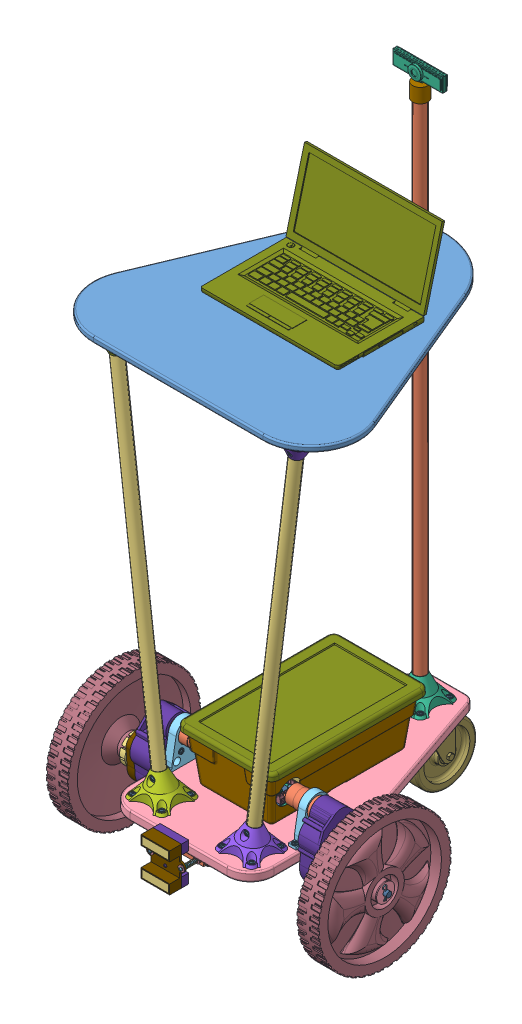
SolidWorks assembly Layla, configuration Default. Lengths in mm. (continued)
Components (placement in the parent): (continued)
- Charger-1: Charger [Default] at (-0.0002 -30.6395 1534.0575) x (1 0 0.000005) z (-0.000005 0 1) size (116 80 70.35)
  - Charger_Back-1: Charger_Back [Default] at (-18.6044 2.3885 -23.0376) size (60 80 15)
  - Charger_Front_1-1: Charger_Front_1 [Default] at (-2.2754 24.6395 -8.0376) x (1 0 0) z (0 -1 0) size (80 25 80)
  - Charger_Front_2-1: Charger_Front_2 [Default] at (-2.2754 54.6395 -6.0376) x (1 0 0) z (0 -1 0) size (54 22 14)
  - Charger_Front_2-2: Charger_Front_2 [Default] at (-2.2754 -5.3605 15.9624) x (1 0 0) z (0 1 0) size (54 22 14)
  - Charge_Bracket-1: Charge_Bracket [Default] at (0 24.6395 -40.9868) x (1 0 0) z (0 1 0) size (116 10 12)
  - Charge_Plate-1: Charge_Plate [Default] at (-2.2754 -5.3605 16.9624) x (-1 0 0) z (0 -1 0) size (56 24 16)
  - Charge_Plate-2: Charge_Plate [Default] at (-2.2754 54.6395 16.9624) x (1 0 0) z (0 1 0) size (56 24 16)
  - Charger_Washer_10-1: Charger_Washer_10 [Default] at (-32.2754 24.6395 -2.5898) x (1 0 0) z (0 1 0) size (12.57 1.45 12.57)
  - Charger_Bolt_6_(2.0'')-1: Charger_Bolt_6_(2.0'') [Default] at (-32.2754 24.6395 -53.3898) x (0 1 0) z (1 0 0) size (6.6 54.26 6.6)
  - Charger_Nut_6-1: Charger_Nut_6 [Default] at (-32.2754 24.6395 -12.4826) x (0 -1 0) z (-1 0 0) size (7.87 4.45 7.87)
  - Charger_Spring-1: Charger_Spring [Default] at (-32.2754 24.6395 -12.7475) x (0.535047 0.844822 0) z (-0.844822 0.535047 0) size (8.88 22.59 8.88)
  - Charger_Washer_10-2: Charger_Washer_10 [Default] at (-32.2754 24.6395 -35.9868) x (0.916814 0.399313 0) z (0.399313 -0.916814 0) size (12.57 1.45 12.57)
  - Charger_Nut_6-2: Charger_Nut_6 [Default] at (-32.2754 24.6395 -45.9868) x (1 0 0) z (0 1 0) size (7.87 4.45 7.87)
  - Charger_Washer_10-3: Charger_Washer_10 [Default] at (32.2754 24.6395 -35.9868) x (-0.916814 0.399313 0) z (0.399313 0.916814 0) size (12.57 1.45 12.57)
  - Charger_Nut_6-3: Charger_Nut_6 [Default] at (32.2754 24.6395 -45.9868) x (-1 0 0) z (0 -1 0) size (7.87 4.45 7.87)
  - Charger_Spring-2: Charger_Spring [Default] at (32.2754 24.6395 -34.274) x (0.535047 -0.844822 0) z (-0.844822 -0.535047 0) size (8.88 22.59 8.88)
  - Charger_Nut_6-4: Charger_Nut_6 [Default] at (32.2754 24.6395 -12.4826) x (0 -1 0) z (-1 0 0) size (7.87 4.45 7.87)
  - Charger_Bolt_6_(2.0'')-2: Charger_Bolt_6_(2.0'') [Default] at (32.2754 24.6395 -53.3898) x (0 1 0) z (1 0 0) size (6.6 54.26 6.6)
  - Charger_Washer_10-4: Charger_Washer_10 [Default] at (32.2754 24.6395 -2.5898) x (-1 0 0) z (0 -1 0) size (12.57 1.45 12.57)
  - Charger_Bolt_Small-1: Charger_Bolt_Small [Default] at (-2.2754 36.6395 -17.7376) x (1 0 0) z (0 -1 0) size (6.1 16.05 6.1)
  - Charger_Bolt_Small-2: Charger_Bolt_Small [Default] at (-2.2754 12.6395 -17.7376) x (1 0 0) z (0 -1 0) size (6.1 16.05 6.1)
- Screw_8_(0.75'')-42: Screw_8_(0.75'') [Default] at (-52 6.7 1493.0704) x (-1 0 0) z (0 0 1) size (10.85 21.85 10.85)
- Screw_8_(0.75'')-43: Screw_8_(0.75'') [Default] at (52 6.7 1493.071) x (-1 0 0) z (0 0 1) size (10.85 21.85 10.85)
Mates (geometry in assembly coordinates):
- Coincident24: coincident anti-aligned: circle of Layla_Bottom-1; circle of frame_bracket_volcano_back-2
- Coincident25: coincident anti-aligned: circle of Layla_Bottom-1; circle of frame_bracket_volcano_back-2
- Coincident27: coincident anti-aligned: plane of Conduit_Back-1 through (0.0274 19.05 997.2192) normal (0 -1 0); plane of Layla_Bottom-1 through (-101.5998 19.05 1455.2076) normal (0 1 0)
- Concentric21: concentric anti-aligned: circle of Conduit_Back-1; circle of Layla_Bottom-1
- Concentric81: concentric anti-aligned: circle of Layla_Top-1; circle of frame_bracket_volcano_back-1
- Coincident75: coincident anti-aligned: plane of Layla_Top-1 through (0.0268 830.9031 1092.4746) normal (0 -1 0); plane of frame_bracket_volcano_back-1 through (0.0274 830.9031 997.2192) normal (0 1 0)
- Concentric83: concentric anti-aligned: circle of Layla_Top-1; circle of frame_bracket_volcano_back-1
- Coincident80: coincident anti-aligned: axis of Conduit_Back-1 through (0.0274 19.05 997.2192) axis (0 1 0); axis of frame_bracket_volcano_back-1 through (0.0274 809.7628 997.2192) axis (0 -1 0)
- Parallel28: parallel aligned: line of Layla_Top-1 through (-0.0833 830.9031 1505.2246) axis (0 0 -1); line of Layla_Bottom-1 through (0 19.05 1501.2457) axis (0 0 -1)
- Coincident89: coincident anti-aligned: circle of Layla_Bottom-1; circle of motor_bracket-1
- Coincident90: coincident aligned: circle of Layla_Bottom-1; circle of motor_bracket-1
- Coincident91: coincident anti-aligned: circle of Layla_Bottom-1; circle of motor_bracket-2
- Coincident92: coincident aligned: circle of Layla_Bottom-1; circle of motor_bracket-2
- Concentric84: concentric aligned: circle of Conduit_Back-1; circle of Camera_Bracket-1
- Coincident94: coincident anti-aligned: plane of Conduit_Back-1 through (0.0274 1136.65 997.2192) normal (0 1 0); plane of Camera_Bracket-1 through (0.0274 1136.65 997.2192) normal (0 -1 0)
- Concentric86: concentric aligned: circle of Layla_Bottom-1; circle of frame_bracket_volcano_right-1
- Concentric87: concentric aligned: circle of Layla_Bottom-1; circle of frame_bracket_volcano_right-1
- Coincident104: coincident anti-aligned: plane of Layla_Bottom-1 through (-101.5998 19.05 1455.2076) normal (0 1 0); plane of frame_bracket_volcano_right-1 through (-94.2631 19.05 1445.5525) normal (0 -1 0)
- Concentric88: concentric aligned: circle of Layla_Bottom-1; circle of frame_bracket_volcano_left-1
- Concentric89: concentric aligned: circle of Layla_Bottom-1; circle of frame_bracket_volcano_left-1
- Coincident105: coincident anti-aligned: plane of Layla_Bottom-1 through (-101.5998 19.05 1455.2076) normal (0 1 0); plane of frame_bracket_volcano_left-1 through (94.2631 19.05 1445.5525) normal (0 -1 0)
- Coincident106: coincident aligned: circle of Conduit_Front-1; circle of frame_bracket_volcano_left-1
- Coincident107: coincident aligned: circle of Conduit_Front-2; circle of frame_bracket_volcano_right-1
- Coincident108: coincident anti-aligned: axis of Conduit_Front-2 through (-94.5769 21.6058 1445.5526) axis (-0.121869 0.992546 0.000001); axis of frame_bracket_volcano_right-1 through (-100.3565 68.6773 1445.5526) axis (0.121869 -0.992546 -0.000001)
- Coincident109: coincident anti-aligned: axis of Conduit_Front-1 through (94.5769 21.6058 1445.5526) axis (0.121869 0.992546 0.000001); axis of frame_bracket_volcano_left-1 through (100.3565 68.6773 1445.5526) axis (-0.121869 -0.992546 -0.000001)
- Coincident110: coincident anti-aligned: circle of Conduit_Front-2; circle of frame_bracket_volcano_right-2
- Coincident111: coincident aligned: axis of Conduit_Front-2 through (-94.5769 21.6058 1445.5526) axis (-0.121869 0.992546 0.000001); axis of frame_bracket_volcano_right-2 through (-187.8526 781.2758 1445.5534) axis (-0.121869 0.992546 0.000001)
- Coincident112: coincident anti-aligned: circle of Conduit_Front-1; circle of frame_bracket_volcano_left-2
- Coincident113: coincident aligned: axis of Conduit_Front-1 through (94.5769 21.6058 1445.5526) axis (0.121869 0.992546 0.000001); axis of frame_bracket_volcano_left-2 through (187.8526 781.2758 1445.5534) axis (0.121869 0.992546 0.000001)
- Coincident114: coincident anti-aligned: plane of Layla_Top-1 through (0.0268 830.9031 1092.4746) normal (0 -1 0); plane of frame_bracket_volcano_left-2 through (193.9461 830.9031 1445.5534) normal (0 1 0)
- Concentric91: concentric aligned: circle of Axle_7_16-2; circle of axle_bracket_7_16-1
- Parallel34: parallel anti-aligned: plane of Layla_Bottom-1 through (-101.5998 0 1455.2076) normal (0 -1 0); plane of axle_bracket_7_16-1 through (74.0819 -2.9787 1334.7553) normal (0 1 0)
- Coincident124: coincident anti-aligned: line of Layla_Bottom-1 through (36.5029 0 951.0085) axis (-0.000005 0 1); line of Caster Part-1 through (36.5024 0 1043.0085) axis (0.000005 0 -1)
- Coincident125: coincident aligned: line of Layla_Bottom-1 through (-36.4971 0 951.0081) axis (-0.000005 0 1); line of Caster Part-1 through (-36.4971 0 951.0081) axis (-0.000005 0 1)
- Coincident126: coincident aligned: line of Layla_Bottom-1 through (36.5029 0 951.0085) axis (-1 0 -0.000005); line of Caster Part-1 through (36.5029 0 951.0085) axis (-1 0 -0.000005)
- Coincident188: coincident aligned: plane of Laptop-2 through (0 841.3074 1314.5854) normal (1 0 0); plane of assembly through (0 0 0) normal (1 0 0)
- Coincident189: coincident anti-aligned: plane of Layla_Top-1 through (0.0268 843.6031 1092.4746) normal (0 1 0); plane of Laptop-2 through (220.359 843.6031 1126.8803) normal (0 -1 0)
- Coincident191: coincident anti-aligned: plane of Caster Part-1 through (176.8474 -3.048 944.9392) normal (0 -1 0); plane of Screw_8_(0.75'')-1 through (-22.2101 -3.048 1035.0706) normal (0 1 0)
- Concentric140: concentric aligned: circle of Caster Part-1; circle of Screw_8_(0.75'')-1
- Parallel92: parallel anti-aligned: plane of Screw_8_(0.75'')-1; plane of assembly through (0 0 0) normal (1 0 0)
- Coincident193: coincident anti-aligned: plane of Caster Part-1 through (176.8474 -3.048 944.9392) normal (0 -1 0); plane of Screw_8_(0.75'')-2 through (22.2149 -3.048 1035.0709) normal (0 1 0)
- Parallel93: parallel anti-aligned: plane of Screw_8_(0.75'')-2; plane of assembly through (0 0 0) normal (1 0 0)
- Concentric141: concentric anti-aligned: circle of Caster Part-1; circle of Screw_8_(0.75'')-2
- Coincident194: coincident anti-aligned: plane of Caster Part-1 through (176.8474 -3.048 944.9392) normal (0 -1 0); plane of Screw_8_(0.75'')-3 through (22.2153 -3.048 958.9459) normal (0 1 0)
- Parallel94: parallel anti-aligned: plane of Screw_8_(0.75'')-3; plane of assembly through (0 0 0) normal (1 0 0)
- Concentric142: concentric aligned: circle of Caster Part-1; circle of Screw_8_(0.75'')-3
- Coincident195: coincident anti-aligned: plane of Caster Part-1 through (176.8474 -3.048 944.9392) normal (0 -1 0); plane of Screw_8_(0.75'')-4 through (-22.2097 -3.048 958.9456) normal (0 1 0)
- Parallel95: parallel anti-aligned: plane of Screw_8_(0.75'')-4; plane of assembly through (0 0 0) normal (1 0 0)
- Concentric143: concentric anti-aligned: circle of Caster Part-1; circle of Screw_8_(0.75'')-4
- Parallel96: parallel anti-aligned: plane of Screw_8_(0.75'')-5; plane of assembly through (0 0 0) normal (1 0 0)
- Coincident196: coincident anti-aligned: plane of axle_bracket_7_16-1 through (82.3318 -5.1787 1347.2554) normal (0 -1 0); plane of Screw_8_(0.75'')-5 through (82.3319 -5.1787 1341.0054) normal (0 1 0)
- Concentric144: concentric aligned: circle of axle_bracket_7_16-1; circle of Screw_8_(0.75'')-5
- Parallel98: parallel anti-aligned: plane of Screw_8_(0.75'')-7; plane of assembly through (0 0 0) normal (1 0 0)
- Coincident198: coincident anti-aligned: plane of axle_bracket_7_16-2 through (-82.3304 -5.1787 1375.5668) normal (0 -1 0); plane of Screw_8_(0.75'')-7 through (-82.3303 -5.1787 1373.3168) normal (0 1 0)
- Concentric146: concentric anti-aligned: circle of axle_bracket_7_16-2; circle of Screw_8_(0.75'')-7
- Parallel100: parallel anti-aligned: plane of Screw_8_(0.75'')-9 through (124.3148 10.35 1475.6049) normal (-1 0 0); plane of assembly through (0 0 0) normal (1 0 0)
- Coincident200: coincident anti-aligned: plane of frame_bracket_volcano_left-1 through (124.3148 23.05 1477.8549) normal (0 1 0); plane of Screw_8_(0.75'')-9 through (124.3148 23.05 1475.6049) normal (0 -1 0)
- Concentric148: concentric aligned: circle of frame_bracket_volcano_left-1; circle of Screw_8_(0.75'')-9
- Parallel101: parallel anti-aligned: plane of Screw_8_(0.75'')-10 through (124.3154 10.35 1415.5008) normal (-1 0 0); plane of assembly through (0 0 0) normal (1 0 0)
- Concentric149: concentric aligned: circle of frame_bracket_volcano_left-1; circle of Screw_8_(0.75'')-10
- Coincident202: coincident anti-aligned: plane of frame_bracket_volcano_left-1 through (124.3153 23.05 1417.7508) normal (0 1 0); plane of Screw_8_(0.75'')-10 through (124.3154 23.05 1415.5008) normal (0 -1 0)
- Parallel102: parallel anti-aligned: plane of Screw_8_(0.75'')-11 through (64.2113 10.35 1415.5002) normal (-1 0 0); plane of assembly through (0 0 0) normal (1 0 0)
- Concentric150: concentric aligned: circle of frame_bracket_volcano_left-1; circle of Screw_8_(0.75'')-11
- Coincident204: coincident anti-aligned: plane of frame_bracket_volcano_left-1 through (64.2113 23.05 1417.7502) normal (0 1 0); plane of Screw_8_(0.75'')-11 through (64.2113 23.05 1415.5002) normal (0 -1 0)
- Parallel103: parallel anti-aligned: plane of Screw_8_(0.75'')-12 through (64.2107 10.35 1475.6043) normal (-1 0 0); plane of assembly through (0 0 0) normal (1 0 0)
- Coincident205: coincident anti-aligned: plane of frame_bracket_volcano_left-1 through (64.2107 23.05 1477.8543) normal (0 1 0); plane of Screw_8_(0.75'')-12 through (64.2107 23.05 1475.6043) normal (0 -1 0)
- Concentric151: concentric aligned: circle of frame_bracket_volcano_left-1; circle of Screw_8_(0.75'')-12
- Parallel104: parallel anti-aligned: plane of Screw_8_(0.75'')-13 through (-64.2107 10.35 1475.6043) normal (-1 0 0); plane of assembly through (0 0 0) normal (1 0 0)
- Coincident206: coincident anti-aligned: plane of frame_bracket_volcano_right-1 through (-64.2107 23.05 1477.8543) normal (0 1 0); plane of Screw_8_(0.75'')-13 through (-64.2107 23.05 1475.6043) normal (0 -1 0)
- Concentric152: concentric anti-aligned: circle of frame_bracket_volcano_right-1; circle of Screw_8_(0.75'')-13
- Parallel105: parallel anti-aligned: plane of Screw_8_(0.75'')-14 through (-124.3148 10.35 1475.6049) normal (-1 0 0); plane of assembly through (0 0 0) normal (1 0 0)
- Coincident208: coincident anti-aligned: plane of frame_bracket_volcano_right-1 through (-124.3148 23.05 1477.8549) normal (0 1 0); plane of Screw_8_(0.75'')-14 through (-124.3148 23.05 1475.6049) normal (0 -1 0)
- Concentric153: concentric anti-aligned: circle of frame_bracket_volcano_right-1; circle of Screw_8_(0.75'')-14
- Parallel106: parallel anti-aligned: plane of Screw_8_(0.75'')-15 through (-124.3154 10.35 1415.5008) normal (-1 0 0); plane of assembly through (0 0 0) normal (1 0 0)
- Coincident209: coincident anti-aligned: plane of frame_bracket_volcano_right-1 through (-124.3153 23.05 1417.7508) normal (0 1 0); plane of Screw_8_(0.75'')-15 through (-124.3154 23.05 1415.5008) normal (0 -1 0)
- Concentric154: concentric anti-aligned: circle of frame_bracket_volcano_right-1; circle of Screw_8_(0.75'')-15
- Parallel108: parallel anti-aligned: plane of Screw_8_(0.75'')-17 through (-64.2113 10.35 1415.5002) normal (-1 0 0); plane of assembly through (0 0 0) normal (1 0 0)
- Coincident211: coincident anti-aligned: plane of frame_bracket_volcano_right-1 through (-64.2113 23.05 1417.7502) normal (0 1 0); plane of Screw_8_(0.75'')-17 through (-64.2113 23.05 1415.5002) normal (0 -1 0)
- Concentric156: concentric anti-aligned: circle of frame_bracket_volcano_right-1; circle of Screw_8_(0.75'')-17
- Parallel109: parallel anti-aligned: plane of Screw_8_(0.75'')-18 through (-136.3198 11.314 1395.7818) normal (-1 0 0); plane of assembly through (0 0 0) normal (1 0 0)
- Coincident212: coincident anti-aligned: plane of motor_bracket-2 through (-136.3143 24.014 1395.7771) normal (0 1 0); plane of Screw_8_(0.75'')-18 through (-136.3198 24.014 1395.7818) normal (0 -1 0)
- Concentric157: concentric anti-aligned: circle of motor_bracket-2; circle of Screw_8_(0.75'')-18
- Parallel110: parallel anti-aligned: plane of Screw_8_(0.75'')-19 through (-136.3202 11.314 1318.2818) normal (-1 0 0); plane of assembly through (0 0 0) normal (1 0 0)
- Coincident213: coincident anti-aligned: plane of motor_bracket-2 through (-136.3147 24.014 1318.2866) normal (0 1 0); plane of Screw_8_(0.75'')-19 through (-136.3202 24.014 1318.2818) normal (0 -1 0)
- Concentric158: concentric aligned: circle of motor_bracket-2; circle of Screw_8_(0.75'')-19
- Parallel111: parallel anti-aligned: plane of Screw_8_(0.75'')-20 through (136.3198 11.314 1395.7818) normal (-1 0 0); plane of assembly through (0 0 0) normal (1 0 0)
- Coincident214: coincident anti-aligned: plane of motor_bracket-1 through (136.3143 24.014 1395.7771) normal (0 1 0); plane of Screw_8_(0.75'')-20 through (136.3198 24.014 1395.7818) normal (0 -1 0)
- Concentric159: concentric aligned: circle of motor_bracket-1; circle of Screw_8_(0.75'')-20
- Parallel112: parallel anti-aligned: plane of Screw_8_(0.75'')-21 through (136.3202 11.314 1318.2818) normal (-1 0 0); plane of assembly through (0 0 0) normal (1 0 0)
- Coincident215: coincident anti-aligned: plane of motor_bracket-1 through (136.3147 24.014 1318.2866) normal (0 1 0); plane of Screw_8_(0.75'')-21 through (136.3202 24.014 1318.2818) normal (0 -1 0)
- Concentric160: concentric anti-aligned: circle of motor_bracket-1; circle of Screw_8_(0.75'')-21
- Parallel113: parallel anti-aligned: plane of Screw_8_(0.75'')-22 through (30.0513 10.35 1027.3271) normal (-1 0 0); plane of assembly through (0 0 0) normal (1 0 0)
- Coincident216: coincident anti-aligned: plane of frame_bracket_volcano_back-2 through (30.0491 23.05 1025.0771) normal (0 1 0); plane of Screw_8_(0.75'')-22 through (30.0513 23.05 1027.3271) normal (0 -1 0)
- Concentric161: concentric anti-aligned: circle of frame_bracket_volcano_back-2; circle of Screw_8_(0.75'')-22
- Parallel114: parallel anti-aligned: plane of Screw_8_(0.75'')-23 through (29.9912 10.35 967.223) normal (-1 0 0); plane of assembly through (0 0 0) normal (1 0 0)
- Coincident217: coincident anti-aligned: plane of frame_bracket_volcano_back-2 through (29.9889 23.05 964.973) normal (0 1 0); plane of Screw_8_(0.75'')-23 through (29.9912 23.05 967.223) normal (0 -1 0)
- Concentric162: concentric anti-aligned: circle of frame_bracket_volcano_back-2; circle of Screw_8_(0.75'')-23
- Parallel115: parallel anti-aligned: plane of Screw_8_(0.75'')-24 through (-30.1129 10.35 967.2832) normal (-1 0 0); plane of assembly through (0 0 0) normal (1 0 0)
- Coincident218: coincident anti-aligned: plane of frame_bracket_volcano_back-2 through (-30.1151 23.05 965.0332) normal (0 1 0); plane of Screw_8_(0.75'')-24 through (-30.1129 23.05 967.2832) normal (0 -1 0)
- Concentric163: concentric anti-aligned: circle of frame_bracket_volcano_back-2; circle of Screw_8_(0.75'')-24
- Parallel116: parallel anti-aligned: plane of Screw_8_(0.75'')-25 through (-30.0527 10.35 1027.3872) normal (-1 0 0); plane of assembly through (0 0 0) normal (1 0 0)
- Coincident219: coincident anti-aligned: plane of frame_bracket_volcano_back-2 through (-30.055 23.05 1025.1372) normal (0 1 0); plane of Screw_8_(0.75'')-25 through (-30.0527 23.05 1027.3872) normal (0 -1 0)
- Concentric164: concentric anti-aligned: circle of frame_bracket_volcano_back-2; circle of Screw_8_(0.75'')-25
- Coincident222: coincident anti-aligned: plane of frame_bracket_volcano_back-2 through (-0.0446 50.3 983.4551) normal (-0.001001 0 -0.999999); plane of Screw_8_(0.75'')-28 through (-0.0446 56.55 983.4551) normal (0.001001 0 0.999999)
- Concentric167: concentric aligned: circle of frame_bracket_volcano_back-2; circle of Screw_8_(0.75'')-28
- Parallel121: parallel aligned: plane of Layla_Bottom-1 through (-101.5998 19.05 1455.2076) normal (0 1 0); plane of Screw_8_(0.75'')-28
- Coincident225: coincident anti-aligned: plane of frame_bracket_volcano_left-1 through (103.0472 51.655 1459.4026) normal (-0.000009 0 1); plane of Screw_8_(0.75'')-29 through (98.833 56.2705 1459.4026) normal (0.000009 0 -1)
- Concentric168: concentric anti-aligned: circle of frame_bracket_volcano_left-1; circle of Screw_8_(0.75'')-29
- Parallel122: parallel aligned: plane of Layla_Bottom-1 through (-101.5998 19.05 1455.2076) normal (0 1 0); plane of Screw_8_(0.75'')-29
- Parallel123: parallel aligned: plane of Layla_Bottom-1 through (-101.5998 19.05 1455.2076) normal (0 1 0); plane of Screw_8_(0.75'')-30
- Coincident226: coincident anti-aligned: plane of frame_bracket_volcano_right-1 through (-103.0472 51.655 1459.4026) normal (0.000009 0 1); plane of Screw_8_(0.75'')-30 through (-98.833 56.2705 1459.4026) normal (-0.000009 0 -1)
- Concentric169: concentric aligned: circle of frame_bracket_volcano_right-1; circle of Screw_8_(0.75'')-30
- Parallel125: parallel aligned: plane of Layla_Top-1 through (0.0268 830.9031 1092.4746) normal (0 -1 0); plane of Screw_8_(0.75'')-32
- Coincident228: coincident anti-aligned: plane of frame_bracket_volcano_right-2 through (-185.1617 798.2982 1459.4033) normal (0.000009 0 1); plane of Screw_8_(0.75'')-32 through (-189.3759 793.6826 1459.4034) normal (-0.000009 0 -1)
- Concentric170: concentric aligned: circle of frame_bracket_volcano_right-2; circle of Screw_8_(0.75'')-32
- Coincident229: coincident anti-aligned: plane of frame_bracket_volcano_left-2 through (185.1617 798.2982 1459.4033) normal (-0.000009 0 1); plane of Screw_8_(0.75'')-33 through (189.3759 793.6826 1459.4034) normal (0.000009 0 -1)
- Concentric171: concentric anti-aligned: circle of frame_bracket_volcano_left-2; circle of Screw_8_(0.75'')-33
- Parallel126: parallel aligned: plane of Layla_Bottom-1 through (-101.5998 19.05 1455.2076) normal (0 1 0); plane of Screw_8_(0.75'')-33
- Parallel127: parallel aligned: plane of Layla_Bottom-1 through (-101.5998 19.05 1455.2076) normal (0 1 0); plane of Screw_8_(0.75'')-34
- Coincident230: coincident anti-aligned: plane of frame_bracket_volcano_back-1 through (0.0118 799.6531 983.3692) normal (-0.00113 0 -0.999999); plane of Screw_8_(0.75'')-34 through (0.0118 793.4031 983.3692) normal (0.00113 0 0.999999)
- Concentric172: concentric aligned: circle of frame_bracket_volcano_back-1; circle of Screw_8_(0.75'')-34
- Coincident245: coincident anti-aligned: plane of frame_bracket_volcano_left-2 through (223.9978 826.9031 1477.8557) normal (0 -1 0); plane of Screw_8_(0.5'')-1 through (223.9979 826.9031 1475.6057) normal (0 1 0)
- Concentric185: concentric anti-aligned: circle of frame_bracket_volcano_left-2; circle of Screw_8_(0.5'')-1
- Parallel143: parallel anti-aligned: plane of Screw_8_(0.5'')-1; plane of Layla_Top-1 through (-0.0562 830.9031 1403.6246) normal (1 0 0.000267)
- Coincident247: coincident anti-aligned: plane of frame_bracket_volcano_left-2 through (223.9978 826.9031 1477.8557) normal (0 -1 0); plane of Screw_8_(0.5'')-2 through (163.8938 826.9031 1475.6052) normal (0 1 0)
- Concentric186: concentric anti-aligned: circle of frame_bracket_volcano_left-2; circle of Screw_8_(0.5'')-2
- Parallel144: parallel anti-aligned: plane of Layla_Top-1 through (-0.0562 830.9031 1403.6246) normal (1 0 0.000267); plane of Screw_8_(0.5'')-2
- Coincident248: coincident anti-aligned: plane of frame_bracket_volcano_left-2 through (223.9978 826.9031 1477.8557) normal (0 -1 0); plane of Screw_8_(0.5'')-3 through (163.8943 826.9031 1415.5011) normal (0 1 0)
- Parallel145: parallel anti-aligned: plane of Layla_Top-1 through (-0.0562 830.9031 1403.6246) normal (1 0 0.000267); plane of Screw_8_(0.5'')-3
- Concentric187: concentric anti-aligned: circle of frame_bracket_volcano_left-2; circle of Screw_8_(0.5'')-3
- Coincident249: coincident anti-aligned: plane of frame_bracket_volcano_left-2 through (223.9978 826.9031 1477.8557) normal (0 -1 0); plane of Screw_8_(0.5'')-4 through (223.9984 826.9031 1415.5017) normal (0 1 0)
- Parallel146: parallel anti-aligned: plane of Layla_Top-1 through (-0.0562 830.9031 1403.6246) normal (1 0 0.000267); plane of Screw_8_(0.5'')-4
- Concentric188: concentric anti-aligned: circle of frame_bracket_volcano_left-2; circle of Screw_8_(0.5'')-4
- Coincident251: coincident anti-aligned: plane of frame_bracket_volcano_right-2 through (-163.8937 826.9031 1477.8552) normal (0 -1 0); plane of Screw_8_(0.5'')-6 through (-163.8938 826.9031 1475.6052) normal (0 1 0)
- Concentric190: concentric aligned: circle of frame_bracket_volcano_right-2; circle of Screw_8_(0.5'')-6
- Parallel148: parallel anti-aligned: plane of Layla_Top-1 through (-0.0562 830.9031 1403.6246) normal (1 0 0.000267); plane of Screw_8_(0.5'')-6
- Coincident252: coincident anti-aligned: plane of frame_bracket_volcano_left-2 through (223.9978 826.9031 1477.8557) normal (0 -1 0); plane of Screw_8_(0.5'')-7 through (-223.9979 826.9031 1475.6057) normal (0 1 0)
- Parallel149: parallel anti-aligned: plane of Layla_Top-1 through (-0.0562 830.9031 1403.6246) normal (1 0 0.000267); plane of Screw_8_(0.5'')-7
- Concentric191: concentric aligned: circle of frame_bracket_volcano_right-2; circle of Screw_8_(0.5'')-7
- Coincident253: coincident anti-aligned: plane of frame_bracket_volcano_left-2 through (223.9978 826.9031 1477.8557) normal (0 -1 0); plane of Screw_8_(0.5'')-8 through (-223.9984 826.9031 1415.5017) normal (0 1 0)
- Parallel150: parallel anti-aligned: plane of Layla_Top-1 through (-0.0562 830.9031 1403.6246) normal (1 0 0.000267); plane of Screw_8_(0.5'')-8
- Concentric192: concentric aligned: circle of frame_bracket_volcano_right-2; circle of Screw_8_(0.5'')-8
- Coincident254: coincident anti-aligned: plane of frame_bracket_volcano_left-2 through (223.9978 826.9031 1477.8557) normal (0 -1 0); plane of Screw_8_(0.5'')-9 through (-163.8943 826.9031 1415.5011) normal (0 1 0)
- Parallel151: parallel anti-aligned: plane of Layla_Top-1 through (-0.0562 830.9031 1403.6246) normal (1 0 0.000267); plane of Screw_8_(0.5'')-9
- Concentric193: concentric aligned: circle of frame_bracket_volcano_right-2; circle of Screw_8_(0.5'')-9
- Parallel152: parallel anti-aligned: plane of Layla_Top-1 through (-0.0562 830.9031 1403.6246) normal (1 0 0.000267); plane of Screw_8_(0.5'')-10
- Coincident255: coincident anti-aligned: plane of frame_bracket_volcano_back-1 through (30.1108 826.9031 1024.9873) normal (0 -1 0); plane of Screw_8_(0.5'')-10 through (30.1134 826.9031 1027.2373) normal (0 1 0)
- Concentric194: concentric aligned: circle of frame_bracket_volcano_back-1; circle of Screw_8_(0.5'')-10
- Parallel153: parallel anti-aligned: plane of Layla_Top-1 through (-0.0562 830.9031 1403.6246) normal (1 0 0.000267); plane of Screw_8_(0.5'')-11
- Coincident257: coincident anti-aligned: plane of frame_bracket_volcano_back-1 through (-29.9932 826.9031 1025.0552) normal (0 -1 0); plane of Screw_8_(0.5'')-11 through (-29.9907 826.9031 1027.3052) normal (0 1 0)
- Concentric195: concentric aligned: circle of frame_bracket_volcano_back-1; circle of Screw_8_(0.5'')-11
- Parallel154: parallel anti-aligned: plane of Layla_Top-1 through (-0.0562 830.9031 1403.6246) normal (1 0 0.000267); plane of Screw_8_(0.5'')-12
- Coincident258: coincident anti-aligned: plane of frame_bracket_volcano_back-1 through (-30.0611 826.9031 964.9511) normal (0 -1 0); plane of Screw_8_(0.5'')-12 through (-30.0586 826.9031 967.2011) normal (0 1 0)
- Concentric196: concentric aligned: circle of frame_bracket_volcano_back-1; circle of Screw_8_(0.5'')-12
- Parallel155: parallel anti-aligned: plane of Layla_Top-1 through (-0.0562 830.9031 1403.6246) normal (1 0 0.000267); plane of Screw_8_(0.5'')-13
- Coincident259: coincident anti-aligned: plane of frame_bracket_volcano_back-1 through (30.0429 826.9031 964.8832) normal (0 -1 0); plane of Screw_8_(0.5'')-13 through (30.0455 826.9031 967.1332) normal (0 1 0)
- Concentric197: concentric aligned: circle of frame_bracket_volcano_back-1; circle of Screw_8_(0.5'')-13
- Concentric201: concentric anti-aligned: circle of Axle_7_16-2; circle of Washer_7_16-1
- Lock5: lock: unknown of Layla_Top-1; unknown of Laptop-2
- Concentric219: concentric aligned: cylinder of motor_bracket-1 through (144.32 74.2738 1357.1619) axis (-1 0 -0.000005) radius 19.67; cylinder of Peg_Perego_Gearbox-1/Peg_Perego_Gearbox_Motor-1 through (84.611 74.2738 1357.1616) axis (-1 0 -0.000005) radius 17.9705
- Concentric220: concentric anti-aligned: cylinder of Axle_7_16-2 through (294.6408 -8.865 1357.1626) axis (-1 0 -0.000005) radius 5.5563; cylinder of Peg_Perego_Gearbox-1/Peg_Perego_Gearbox_Bottom-1 through (150.8133 -8.865 1357.1619) axis (1 0 0.000005) radius 5.5563
- Coincident268: coincident anti-aligned: plane of Layla_Bottom-1 through (150.8127 19.05 1455.209) normal (1 0 0.000005); plane of Peg_Perego_Gearbox-1/Peg_Perego_Gearbox_Bottom-1 through (150.8133 19.2348 1356.1331) normal (-1 0 -0.000005)
- Coincident271: coincident anti-aligned: plane of Layla_Bottom-1 through (-150.8123 19.05 1455.2074) normal (-1 0 -0.000005); plane of Peg_Perego_Gearbox-8/Peg_Perego_Gearbox_Bottom-1 through (-150.8117 19.2396 1358.0487) normal (1 0 0.000005)
- Concentric225: concentric aligned: cylinder of Axle_7_16-2 through (294.6408 -8.865 1357.1626) axis (-1 0 -0.000005) radius 5.5563; cylinder of Peg_Perego_Gearbox-8/Peg_Perego_Gearbox_Big_Gear-1 through (-194.7537 -8.865 1357.16) axis (-1 0 -0.000005) radius 5.5563
- Parallel161: parallel aligned: plane of Layla_Bottom-1 through (0.0001 0 1480.0562) normal (-0.000005 0 1); plane of Peg_Perego_Gearbox-1
- Lock6: lock: unknown of motor_bracket-2; unknown of ?
- Coincident276: coincident aligned: plane of Layla_Bottom-1 through (0.0001 0 1480.0562) normal (1 0 0.000005); plane of Axle_7_16-2 through (0.0008 -8.865 1357.1611) normal (1 0 0.000005)
- Concentric226: concentric aligned: cylinder of Axle_7_16-2 through (294.6408 -8.865 1357.1627) axis (-1 0 -0.000005) radius 5.5563; circle of 11in_barbie_mower-1
- Coincident278: coincident anti-aligned: plane of Peg_Perego_Gearbox-1/Peg_Perego_Gearbox_Big_Gear-1 through (229.8326 16.6536 1360.7497) normal (0.000001 0.992561 -0.121745); plane of 11in_barbie_mower-1 through (209.5086 16.6536 1360.7496) normal (-0.000001 -0.992561 0.121745)
- Coincident279: coincident anti-aligned: plane of Peg_Perego_Gearbox-1/Peg_Perego_Gearbox_Big_Gear-1 through (229.8327 -8.865 1357.1623) normal (1 0 0.000005); plane of 11in_barbie_mower-1 through (229.8327 -8.865 1357.1623) normal (-1 0 -0.000005)
- Coincident281: coincident anti-aligned: plane of 11in_Mower_Wheel-5 through (231.3567 -8.865 1357.1623) normal (-1 0 -0.000005); plane of 11in_barbie_mower-1 through (231.3567 -8.865 1357.1623) normal (1 0 0.000005)
- Concentric227: concentric anti-aligned: circle of Axle_7_16-2; circle of 11in_Mower_Wheel-5
- Concentric229: concentric aligned: cylinder of Axle_7_16-2 through (294.6408 -8.865 1357.1627) axis (-1 0 -0.000005) radius 5.5563; cylinder of 11in_barbie_mower-3 through (-229.8311 -8.865 1357.1599) axis (-1 0 -0.000005) radius 5.5563
- Coincident285: coincident anti-aligned: plane of Peg_Perego_Gearbox-8/Peg_Perego_Gearbox_Big_Gear-1 through (-229.8311 16.6353 1353.445) normal (-0.000001 0.993157 0.116786); plane of 11in_barbie_mower-3 through (-209.5072 15.078 1366.6889) normal (0.000001 -0.993157 -0.116786)
- Coincident286: coincident anti-aligned: plane of Peg_Perego_Gearbox-8/Peg_Perego_Gearbox_Big_Gear-1 through (-229.8311 -8.865 1357.1599) normal (-1 0 -0.000005); plane of 11in_barbie_mower-3 through (-229.8311 -8.865 1357.1599) normal (1 0 0.000005)
- Coincident287: coincident anti-aligned: plane of 11in_barbie_mower-3 through (-231.3551 -8.865 1357.1599) normal (-1 0 -0.000005); plane of 11in_Mower_Wheel-6 through (-231.3551 -8.865 1357.1599) normal (1 0 0.000005)
- Concentric230: concentric anti-aligned: cylinder of Axle_7_16-2 through (294.6408 -8.865 1357.1627) axis (-1 0 -0.000005) radius 5.5563; cylinder of 11in_Mower_Wheel-6 through (-152.9728 -8.865 1357.1603) axis (1 0 0.000005) radius 5.5563
- Coincident288: coincident anti-aligned: plane of 11in_Mower_Wheel-6 through (-285.3301 -8.865 1357.1596) normal (-1 0 -0.000005); plane of Washer_7_16-1 through (-285.3301 -8.865 1357.1596) normal (1 0 0.000005)
- Concentric231: concentric aligned: cylinder of Axle_7_16-2 through (294.6408 -8.865 1357.1627) axis (-1 0 -0.000005) radius 5.5563; cylinder of Washer_7_16-2 through (285.3317 -8.865 1357.1626) axis (-1 0 -0.000005) radius 5.5563
- Coincident289: coincident anti-aligned: plane of 11in_Mower_Wheel-5 through (285.3317 -8.865 1357.1626) normal (1 0 0.000005); plane of Washer_7_16-2 through (285.3317 -8.865 1357.1626) normal (-1 0 -0.000005)
- Concentric232: concentric anti-aligned: cylinder of Axle_7_16-2 through (288.7988 -15.7178 1357.4306) axis (0 0.999236 -0.039071) radius 0.762; cylinder of Hair Pin Cotter Pin-1 through (288.7988 3.2301 1356.6897) axis (0 -0.999236 0.039071) radius 0.7493
- Parallel162: parallel anti-aligned: plane of Axle_7_16-2 through (0.0008 -8.865 1357.1611) normal (1 0 0.000005); plane of Hair Pin Cotter Pin-1
- Lock7: lock: unknown of Washer_7_16-2; unknown of Hair Pin Cotter Pin-1
- Concentric233: concentric anti-aligned: cylinder of Axle_7_16-2 through (-288.7972 -15.7178 1357.4275) axis (0 0.999236 -0.039071) radius 0.762; cylinder of Hair Pin Cotter Pin-2 through (-288.7972 3.5227 1356.6752) axis (0 -0.999236 0.039071) radius 0.7493
- Parallel163: parallel anti-aligned: plane of Axle_7_16-2 through (0.0008 -8.865 1357.1611) normal (1 0 0.000005); plane of Hair Pin Cotter Pin-2
- Lock8: lock: unknown of Layla_Bottom-1; unknown of Hair Pin Cotter Pin-2
- Parallel164: parallel anti-aligned: plane of Screw_8_(0.75'')-36; plane of assembly through (0 0 0) normal (1 0 0)
- Concentric234: concentric anti-aligned: circle of axle_bracket_7_16-1; circle of Screw_8_(0.75'')-36
- Coincident292: coincident anti-aligned: plane of axle_bracket_7_16-1 through (82.3317 -5.1787 1375.5678) normal (0 -1 0); plane of Screw_8_(0.75'')-36 through (82.3317 -5.1787 1373.3178) normal (0 1 0)
- Parallel165: parallel anti-aligned: plane of Screw_8_(0.75'')-37; plane of assembly through (0 0 0) normal (1 0 0)
- Concentric235: concentric aligned: circle of axle_bracket_7_16-2; circle of Screw_8_(0.75'')-37
- Coincident293: coincident anti-aligned: plane of axle_bracket_7_16-2 through (-82.3302 -5.1787 1347.2544) normal (0 -1 0); plane of Screw_8_(0.75'')-37 through (-82.3302 -5.1787 1341.0044) normal (0 1 0)
- Concentric236: concentric anti-aligned: circle of motor_bracket-2; circle of Screw_8_(0.75'')-38
- Coincident294: coincident anti-aligned: plane of motor_bracket-2 through (-128.32 74.8867 1357.0318) normal (1 0 -0.000005); plane of Screw_8_(0.75'')-38 through (-128.3199 47.7688 1371.1468) normal (-1 0 0.000005)
- Parallel166: parallel anti-aligned: plane of motor_bracket-2; plane of Screw_8_(0.75'')-38
- Parallel167: parallel anti-aligned: plane of motor_bracket-1; plane of Screw_8_(0.75'')-39
- Concentric237: concentric aligned: cylinder of motor_bracket-1 through (144.3201 47.7688 1342.9169) axis (-1 0 -0.000005) radius 4.525; circle of Screw_8_(0.75'')-39
- Coincident295: coincident anti-aligned: plane of motor_bracket-1 through (128.32 74.8867 1357.0318) normal (-1 0 -0.000005); plane of Screw_8_(0.75'')-39 through (128.3201 47.7688 1342.9168) normal (1 0 0.000005)
- Concentric238: concentric aligned: cylinder of Camera_Bracket-1 through (0.0274 1112.519 997.2192) axis (0 1 0) radius 2.54; cylinder of Genius_Webcam-1 through (0.0274 1137.666 997.2192) axis (0 1 0) radius 2.54
- Tangent2: tangent anti-aligned: plane of Camera_Bracket-1 through (0.0274 1142.492 997.2192) normal (0 1 0); cylinder of Genius_Webcam-1 through (-5.6876 1145.9083 997.2192) axis (1 0 0) radius 3.4163
- Parallel168: parallel aligned: plane of Genius_Webcam-1 through (0.0274 1163.8661 993.1679) normal (1 0 0); plane of assembly through (0 0 0) normal (1 0 0)
- Coincident299: coincident anti-aligned: plane of Layla_Bottom-1 through (0.0001 0 1480.0562) normal (1 0 0.000005); plane of ? through (0.0014 61.0324 1233.4944) normal (-1 0 -0.000005)
- Parallel170: parallel aligned: plane of Layla_Bottom-1; plane of ?
- Coincident302: coincident: plane of Layla_Bottom-1 through (-101.5998 19.05 1455.2076) normal (0 1 0); line of ? through (62.6524 19.05 1381.3259) axis (-1 0 -0.000005)
- Lock9: lock: unknown of Layla_Bottom-1; unknown of ?
- Coincident303: coincident aligned: plane of Layla_Bottom-1 through (0.0001 0 1480.0562) normal (1 0 0.000005); plane of Counterweight_Ingot-1
- Coincident304: coincident anti-aligned: plane of Layla_Bottom-1 through (-101.5998 0 1455.2076) normal (0 -1 0); plane of Counterweight_Ingot-1 through (0.0022 0 1072.91) normal (0 1 0)
- Lock10: lock: unknown of Layla_Bottom-1; unknown of Counterweight_Ingot-1
- Parallel172: parallel anti-aligned: plane of Counterweight_Ingot_Screw-1; plane of assembly through (0 0 0) normal (1 0 0)
- Parallel173: parallel anti-aligned: plane of Counterweight_Ingot_Screw-2; plane of assembly through (0 0 0) normal (1 0 0)
- Parallel174: parallel anti-aligned: plane of Layla_Bottom-1 through (-101.5998 19.05 1455.2076) normal (0 1 0); plane of electronics_box-2/Sterilite_Lid-1 through (-6.4052 131.4437 1243.734) normal (0 -1 0)
- Coincident310: coincident: plane of Layla_Bottom-1 through (-101.5998 19.05 1455.2076) normal (0 1 0); line of electronics_box-2/sterilite_box-1 through (-75.6101 19.05 1265.1884) axis (-0.000005 0 1)
- Coincident311: coincident aligned: plane of Layla_Bottom-1 through (0.0001 0 1480.0562) normal (1 0 0.000005); plane of electronics_box-2/Sterilite_Lid-1 through (0.0014 120.6487 1243.7341) normal (1 0 0.000005)
- Coincident314: coincident anti-aligned: plane of motor_bracket-1; plane of ? through (-6.4058 19.0487 1357.0311) normal (0.000005 0 -1)
- Coincident315: coincident anti-aligned: plane of Layla_Bottom-1 through (-101.5998 0 1455.2076) normal (0 -1 0); plane of Charger-1/Charge_Bracket-1 through (58.0001 0 1488.071) normal (0 1 0)
- Coincident316: coincident aligned: plane of Layla_Bottom-1 through (0.0001 0 1480.0562) normal (1 0 0.000005); plane of Charger-1/Charge_Bracket-1
- Parallel177: parallel anti-aligned: plane of Screw_8_(0.75'')-42; plane of assembly through (0 0 0) normal (1 0 0)
- Concentric241: concentric aligned: circle of Charger-1/Charge_Bracket-1; circle of Screw_8_(0.75'')-42
- Coincident318: coincident anti-aligned: plane of Charger-1/Charge_Bracket-1 through (-58 -6 1498.0704) normal (0 -1 0); plane of Screw_8_(0.75'')-42 through (-52 -6 1493.0704) normal (0 1 0)
- Parallel178: parallel anti-aligned: plane of Screw_8_(0.75'')-43; plane of assembly through (0 0 0) normal (1 0 0)
- Concentric242: concentric aligned: circle of Charger-1/Charge_Bracket-1; circle of Screw_8_(0.75'')-43
- Coincident320: coincident anti-aligned: plane of Charger-1/Charge_Bracket-1 through (46 -6 1498.0709) normal (0 -1 0); plane of Screw_8_(0.75'')-43 through (52 -6 1493.071) normal (0 1 0)
- Distance2: distance = 3.175 mm: line of Charger-1/Charge_Bracket-1 through (58 0 1498.071) axis (-1 0 -0.000005); line of Layla_Bottom-1 through (101.6 0 1501.2462) axis (-1 0 -0.000005)
- Concentric243: concentric aligned: circle of Counterweight_Ingot-1; circle of Counterweight_Ingot_Screw-1
- Coincident321: coincident aligned: plane of Counterweight_Ingot-1 through (0.0022 -31.75 1072.91) normal (0 -1 0); circle of Counterweight_Ingot_Screw-1
- Concentric244: concentric aligned: circle of Counterweight_Ingot-1; circle of Counterweight_Ingot_Screw-2
- Coincident322: coincident aligned: plane of Counterweight_Ingot-1 through (0.0022 -31.75 1072.91) normal (0 -1 0); circle of Counterweight_Ingot_Screw-2
